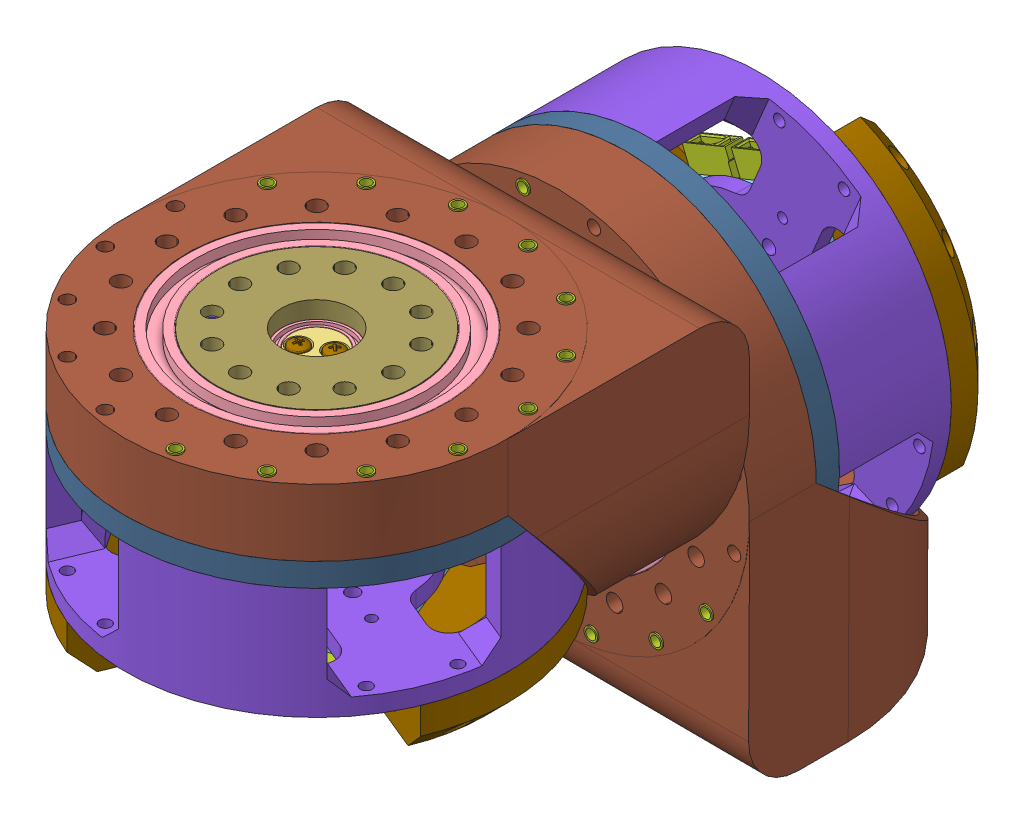
SolidWorks assembly hip, configuration Default. Lengths in mm. (continued)
Components (placement in the parent): (continued)
- Cycloidal_v3-2: Cycloidal_v3 [Default] at (91.3873 -36.6902 -47.4953) x (-0.999985 0.005457 0) z (0.005457 0.999985 0) size (150.25 88 150.25) (continued)
  - foc-motor-controller.step-1: foc-motor-controller.step [Default] at (47.267 33.7573 89.1587) x (-0.382683 0 -0.92388) z (0 -1 0) size (57.23 50 8.13) (continued)
    - RTA0040B.step-1: RTA0040B.step [Default] at (12.5014 -1.6986 1.595) x (-0.707107 -0.707107 0) z (0 0 1) size (6 6 1) (continued)
      - FRAME.step-1: FRAME.step [Default] x (1 0 0) z (0 -1 0) size (6 0.2 6) (continued)
        - SOLID-1.step-1: SOLID-1.step [Default] at origin size (0.4 0.2 0.22)
        - SOLID-2.step-1: SOLID-2.step [Default] at origin size (0.4 0.2 0.22)
        - SOLID-3.step-1: SOLID-3.step [Default] at origin size (0.4 0.2 0.22)
        - SOLID-4.step-1: SOLID-4.step [Default] at origin size (0.4 0.2 0.22)
        - SOLID-5.step-1: SOLID-5.step [Default] at origin size (0.4 0.2 0.22)
        - SOLID-6.step-1: SOLID-6.step [Default] at origin size (0.4 0.2 0.22)
        - SOLID-7.step-1: SOLID-7.step [Default] at origin size (0.4 0.2 0.22)
        - SOLID-8.step-1: SOLID-8.step [Default] at origin size (0.4 0.2 0.22)
        - SOLID-9.step-1: SOLID-9.step [Default] at origin size (0.22 0.2 0.4)
        - SOLID-10.step-1: SOLID-10.step [Default] at origin size (0.22 0.2 0.4)
        - SOLID-11.step-1: SOLID-11.step [Default] at origin size (0.22 0.2 0.4)
        - SOLID-12.step-1: SOLID-12.step [Default] at origin size (0.22 0.2 0.4)
        - SOLID-13.step-1: SOLID-13.step [Default] at origin size (0.22 0.2 0.4)
        - SOLID-14.step-1: SOLID-14.step [Default] at origin size (0.22 0.2 0.4)
        - SOLID-15.step-1: SOLID-15.step [Default] at origin size (0.22 0.2 0.4)
        - SOLID-16.step-1: SOLID-16.step [Default] at origin size (0.22 0.2 0.4)
        - SOLID-17.step-1: SOLID-17.step [Default] at origin size (4.15 0.2 4.15)
        - SOLID-18.step-1: SOLID-18.step [Default] at origin size (0.28 0.1 0.28)
        - SOLID-19.step-1: SOLID-19.step [Default] at origin size (0.28 0.1 0.28)
        - SOLID-20.step-1: SOLID-20.step [Default] at origin size (0.28 0.1 0.28)
        - SOLID-21.step-1: SOLID-21.step [Default] at origin size (0.28 0.1 0.28)
        - SOLID-22.step-1: SOLID-22.step [Default] at origin size (0.4 0.2 0.22)
        - SOLID-23.step-1: SOLID-23.step [Default] at origin size (0.4 0.2 0.22)
        - SOLID-24.step-1: SOLID-24.step [Default] at origin size (0.4 0.2 0.22)
        - SOLID-25.step-1: SOLID-25.step [Default] at origin size (0.4 0.2 0.22)
        - SOLID-26.step-1: SOLID-26.step [Default] at origin size (0.4 0.2 0.22)
        - SOLID-27.step-1: SOLID-27.step [Default] at origin size (0.4 0.2 0.22)
        - SOLID-28.step-1: SOLID-28.step [Default] at origin size (0.4 0.2 0.22)
        - SOLID-29.step-1: SOLID-29.step [Default] at origin size (0.4 0.2 0.22)
        - SOLID-30.step-1: SOLID-30.step [Default] at origin size (0.4 0.2 0.22)
        - SOLID-31.step-1: SOLID-31.step [Default] at origin size (0.4 0.2 0.22)
        - SOLID-32.step-1: SOLID-32.step [Default] at origin size (0.22 0.2 0.4)
        - SOLID-33.step-1: SOLID-33.step [Default] at origin size (0.22 0.2 0.4)
        - SOLID-34.step-1: SOLID-34.step [Default] at origin size (0.22 0.2 0.4)
        - SOLID-35.step-1: SOLID-35.step [Default] at origin size (0.22 0.2 0.4)
        - SOLID-36.step-1: SOLID-36.step [Default] at origin size (0.22 0.2 0.4)
        - SOLID-37.step-1: SOLID-37.step [Default] at origin size (0.22 0.2 0.4)
        - SOLID-38.step-1: SOLID-38.step [Default] at origin size (0.22 0.2 0.4)
        - SOLID-39.step-1: SOLID-39.step [Default] at origin size (0.22 0.2 0.4)
        - SOLID-40.step-1: SOLID-40.step [Default] at origin size (0.22 0.2 0.4)
        - SOLID-41.step-1: SOLID-41.step [Default] at origin size (0.22 0.2 0.4)
        - SOLID-42.step-1: SOLID-42.step [Default] at origin size (0.22 0.2 0.4)
        - SOLID-43.step-1: SOLID-43.step [Default] at origin size (0.22 0.2 0.4)
      - BODY.step-1: BODY.step [Default] at (0 0 0.025) x (1 0 0) z (0 -1 0) size (6 0.97 6)
    - Resonator_SMD_Murata_CSTxExxV-3Pin_3.0x1.1mm.step-1: Resonator_SMD_Murata_CSTxExxV-3Pin_3.0x1.1mm.step [Default] at (1.8 -7 1.595) x (0 1 0) z (0 0 1) size (3.2 1.35 0.9)
    - C_0603_1608Metric.step-1: C_0603_1608Metric.step [Default] at (6.2 -16.8 1.595) x (0 -1 0) z (0 0 1) size (1.6 0.8 0.8)
    - R_0603_1608Metric.step-1: R_0603_1608Metric.step [Default] at (11.8 -7.375 1.595) x (0 1 0) z (0 0 1) size (1.6 0.8 0.45)
    - R_0603_1608Metric.step-2: R_0603_1608Metric.step [Default] at (13.8 -16.8 1.595) x (0 1 0) z (0 0 1) size (1.6 0.8 0.45)
    - R_0603_1608Metric.step-3: R_0603_1608Metric.step [Default] at (18.1 -5.36 1.595) size (1.6 0.8 0.45)
    - C_0603_1608Metric.step-2: C_0603_1608Metric.step [Default] at (2.6 -0.5 1.595) x (0 -1 0) z (0 0 1) size (1.6 0.8 0.8)
    - R_0603_1608Metric.step-4: R_0603_1608Metric.step [Default] at (14.6 -11.3 1.595) x (0 1 0) z (0 0 1) size (1.6 0.8 0.45)
    - L_APV_ANR4020.step-1: L_APV_ANR4020.step [Default] at (22.3 -13.7 1.595) x (0 -1 0) z (0 0 1) size (4.02 4 2)
    - C_0603_1608Metric.step-3: C_0603_1608Metric.step [Default] at (0.3 -12.6 1.595) x (-1 0 0) z (0 0 1) size (1.6 0.8 0.8)
    - C_1206_3216Metric.step-1: C_1206_3216Metric.step [Default] at (15.7 11 1.595) x (0 1 0) z (0 0 1) size (3.2 1.6 1.6)
    - C_0603_1608Metric.step-4: C_0603_1608Metric.step [Default] at (0.3 -9.6 1.595) size (1.6 0.8 0.8)
    - R_0603_1608Metric.step-5: R_0603_1608Metric.step [Default] at (12.3 -16.8 1.595) x (0 1 0) z (0 0 1) size (1.6 0.8 0.45)
    - C_0603_1608Metric.step-5: C_0603_1608Metric.step [Default] at (-0.3 -16.6 1.595) x (0 1 0) z (0 0 1) size (1.6 0.8 0.8)
    - R_0603_1608Metric.step-6: R_0603_1608Metric.step [Default] at (10.9 4.1 1.595) size (1.6 0.8 0.45)
    - C_1206_3216Metric.step-2: C_1206_3216Metric.step [Default] at (6.3 11 1.595) x (0 1 0) z (0 0 1) size (3.2 1.6 1.6)
    - XT30PW_2_2_-M.G.B.step-1: XT30PW_2_2_-M.G.B.step [Default] at (-20.5 9.5 1.595) x (0 -1 0) z (-1 0 0) size (15.5 7.1 12.53)
    - R_0603_1608Metric.step-7: R_0603_1608Metric.step [Default] at (0.3 -11.1 1.595) size (1.6 0.8 0.45)
    - C_0603_1608Metric.step-6: C_0603_1608Metric.step [Default] at (19 -0.4 1.595) x (-0.707107 -0.707107 0) z (0 0 1) size (1.6 0.8 0.8)
    - C_1206_3216Metric.step-3: C_1206_3216Metric.step [Default] at (13.3 11 1.595) x (0 1 0) z (0 0 1) size (3.2 1.6 1.6)
    - R_0603_1608Metric.step-8: R_0603_1608Metric.step [Default] at (10.2 -7.375 1.595) x (0 -1 0) z (0 0 1) size (1.6 0.8 0.45)
    - JST_GH_SM08B-GHS-TB_1x08-1MP_P1.25mm_Horizontal.step-1: JST_GH_SM08B-GHS-TB_1x08-1MP_P1.25mm_Horizontal.step [Default] at (10 -22 1.595) size (13.25 4.95 4.25)
    - C_1206_3216Metric.step-4: C_1206_3216Metric.step [Default] at (-12.3 11 1.595) x (0 1 0) z (0 0 1) size (3.2 1.6 1.6)
    - JST_GH_SM06B-GHS-TB_1x06-1MP_P1.25mm_Horizontal.step-1: JST_GH_SM06B-GHS-TB_1x06-1MP_P1.25mm_Horizontal.step [Default] at (-4.3 -22 1.595) size (10.75 4.95 4.25)
    - C_0603_1608Metric.step-7: C_0603_1608Metric.step [Default] at (7.3 -4.5 1.595) x (-1 0 0) z (0 0 1) size (1.6 0.8 0.8)
    - R_0603_1608Metric.step-9: R_0603_1608Metric.step [Default] at (18.1 -3.86 1.595) x (-1 0 0) z (0 0 1) size (1.6 0.8 0.45)
    - C_1206_3216Metric.step-5: C_1206_3216Metric.step [Default] at (22.6794 -1.2206 1.595) x (0.707107 -0.707107 0) z (0 0 1) size (3.2 1.6 1.6)
    - R_Array_Convex_4x0402.step-1: R_Array_Convex_4x0402.step [Default] at (6.8 -2.5 1.595) size (1 2 0.35)
    - R_0603_1608Metric.step-10: R_0603_1608Metric.step [Default] at (7.7 -16.8 1.595) x (0 -1 0) z (0 0 1) size (1.6 0.8 0.45)
    - C_1206_3216Metric.step-6: C_1206_3216Metric.step [Default] at (8.7 11 1.595) x (0 1 0) z (0 0 1) size (3.2 1.6 1.6)
    - C_0603_1608Metric.step-8: C_0603_1608Metric.step [Default] at (16.1 -11.3 1.595) x (0 1 0) z (0 0 1) size (1.6 0.8 0.8)
    - SOT-23-5.step-1: SOT-23-5.step [Default] at (-3.1 -16.6 1.595) x (-1 0 0) z (0 0 1) size (2.8 2.9 1.55)
    - C_0603_1608Metric.step-9: C_0603_1608Metric.step [Default] at (17.8 -13.6 1.595) size (1.6 0.8 0.8)
    - R_0603_1608Metric.step-11: R_0603_1608Metric.step [Default] at (-11.5 -20.3875 1.595) x (0 -1 0) z (0 0 1) size (1.6 0.8 0.45)
    - C_0603_1608Metric.step-10: C_0603_1608Metric.step [Default] at (-12.4 2.3 1.595) x (0 1 0) z (0 0 1) size (1.6 0.8 0.8)
    - C_1206_3216Metric.step-7: C_1206_3216Metric.step [Default] at (18 11 1.595) x (0 1 0) z (0 0 1) size (3.2 1.6 1.6)
    - R_0603_1608Metric.step-12: R_0603_1608Metric.step [Default] at (-10.8105 -14.9971 1.595) x (-1 0 0) z (0 0 1) size (1.6 0.8 0.45)
    - C_0603_1608Metric.step-11: C_0603_1608Metric.step [Default] at (-13.8 -9.4 1.595) x (-1 0 0) z (0 0 1) size (1.6 0.8 0.8)
    - R_0603_1608Metric.step-13: R_0603_1608Metric.step [Default] at (-23.15 -14.5 1.595) x (-1 0 0) z (0 0 1) size (1.6 0.8 0.45)
    - C_0603_1608Metric.step-12: C_0603_1608Metric.step [Default] at (1.1 -0.2 1.595) x (0 1 0) z (0 0 1) size (1.6 0.8 0.8)
    - D_0805_2012Metric.step-1: D_0805_2012Metric.step [Default] at (22.9 -9.6 1.595) x (0 1 0) z (0 0 1) size (2 1.27 0.8)
    - C_0603_1608Metric.step-13: C_0603_1608Metric.step [Default] at (-7.8 3.775 1.595) x (0 -1 0) z (0 0 1) size (1.6 0.8 0.8)
    - R_0603_1608Metric.step-14: R_0603_1608Metric.step [Default] at (-6.4 -12.825 1.595) x (0 1 0) z (0 0 1) size (1.6 0.8 0.45)
    - L_0603_1608Metric.step-1: L_0603_1608Metric.step [Default] at (-10.1 3 1.595) size (1.6 0.8 0.8)
    - C_0603_1608Metric.step-14: C_0603_1608Metric.step [Default] at (17.9 0.7 1.595) x (-0.707107 -0.707107 0) z (0 0 1) size (1.6 0.8 0.8)
    - HVSSOP-10.step-1: HVSSOP-10.step [Default] at (18.6 -9.6 1.595) x (0 -1 0) z (-1 0 0) size (4.9 1.1 3)
    - C_0603_1608Metric.step-15: C_0603_1608Metric.step [Default] at (7.9 4.1 1.595) x (-1 0 0) z (0 0 1) size (1.6 0.8 0.8)
    - C_0603_1608Metric.step-16: C_0603_1608Metric.step [Default] at (21.1 -9.6 1.595) x (0 -1 0) z (0 0 1) size (1.6 0.8 0.8)
    - R_0603_1608Metric.step-15: R_0603_1608Metric.step [Default] at (-10.8105 -11.9971 1.595) x (-1 0 0) z (0 0 1) size (1.6 0.8 0.45)
    - R_0603_1608Metric.step-16: R_0603_1608Metric.step [Default] at (-18.2 -17.4 1.595) size (1.6 0.8 0.45)
    - C_1206_3216Metric.step-8: C_1206_3216Metric.step [Default] at (-3 11 1.595) x (0 1 0) z (0 0 1) size (3.2 1.6 1.6)
    - R_0603_1608Metric.step-17: R_0603_1608Metric.step [Default] at (-16.9 -20.4 1.595) x (0 -1 0) z (0 0 1) size (1.6 0.8 0.45)
    - R_0603_1608Metric.step-18: R_0603_1608Metric.step [Default] at (-13.3 -20.3875 1.595) x (0 -1 0) z (0 0 1) size (1.6 0.8 0.45)
    - R_0603_1608Metric.step-19: R_0603_1608Metric.step [Default] at (-15.1 -20.3875 1.595) x (0 -1 0) z (0 0 1) size (1.6 0.8 0.45)
    - C_0603_1608Metric.step-17: C_0603_1608Metric.step [Default] at (15.5 -14.4 1.595) x (0 -1 0) z (0 0 1) size (1.6 0.8 0.8)
    - LED_0603_1608Metric.step-1: LED_0603_1608Metric.step [Default] at (-11.5 -23.3875 1.595) x (0 1 0) z (0 0 1) size (1.6 0.8 1.1)
    - C_0805_2012Metric.step-1: C_0805_2012Metric.step [Default] at (19.95 -17 1.595) size (2 1.25 1.25)
    - D_SMB.step-1: D_SMB.step [Default] at (-16.5 11.208 1.595) x (0 -1 0) z (0 0 1) size (5.3 3.55 2.15)
    - C_1206_3216Metric.step-9: C_1206_3216Metric.step [Default] at (-5.3 11 1.595) x (0 1 0) z (0 0 1) size (3.2 1.6 1.6)
    - XT30PW_2_2_-M.G.B.step-2: XT30PW_2_2_-M.G.B.step [Default] at (-20.5 -6.5 1.595) x (0 -1 0) z (-1 0 0) size (15.5 7.1 12.53)
    - C_1206_3216Metric.step-10: C_1206_3216Metric.step [Default] at (1.7 11 1.595) x (0 1 0) z (0 0 1) size (3.2 1.6 1.6)
    - C_1206_3216Metric.step-11: C_1206_3216Metric.step [Default] at (11 11 1.595) x (0 1 0) z (0 0 1) size (3.2 1.6 1.6)
    - C_0603_1608Metric.step-18: C_0603_1608Metric.step [Default] at (-6.3 3.775 1.595) x (0 -1 0) z (0 0 1) size (1.6 0.8 0.8)
    - C_0603_1608Metric.step-19: C_0603_1608Metric.step [Default] at (16.8686 1.7314 1.595) x (0.707107 0.707107 0) z (0 0 1) size (1.6 0.8 0.8)
    - C_0603_1608Metric.step-20: C_0603_1608Metric.step [Default] at (-15.0105 -11.1 1.595) size (1.6 0.8 0.8)
    - C_1206_3216Metric.step-12: C_1206_3216Metric.step [Default] at (-7.7 11 1.595) x (0 1 0) z (0 0 1) size (3.2 1.6 1.6)
    - C_0603_1608Metric.step-21: C_0603_1608Metric.step [Default] at (-18.2 -15.8 1.595) size (1.6 0.8 0.8)
    - C_0603_1608Metric.step-22: C_0603_1608Metric.step [Default] at (-2.1 -11.3 1.595) x (0 -1 0) z (0 0 1) size (1.6 0.8 0.8)
    - C_0603_1608Metric.step-23: C_0603_1608Metric.step [Default] at (-10.8105 -13.4971 1.595) size (1.6 0.8 0.8)
    - C_1206_3216Metric.step-13: C_1206_3216Metric.step [Default] at (4 11 1.595) x (0 1 0) z (0 0 1) size (3.2 1.6 1.6)
    - R_0603_1608Metric.step-20: R_0603_1608Metric.step [Default] at (16 -17.8 1.595) x (0 1 0) z (0 0 1) size (1.6 0.8 0.45)
    - Texas_S-PVSON-N8.step-1: Texas_S-PVSON-N8.step [Default] at (-14.4105 -13.7 1.595) x (-1 0 0) z (0 0 1) size (3 2.98 0.92)
    - C_1206_3216Metric.step-14: C_1206_3216Metric.step [Default] at (21 -2.9 1.595) x (0.707107 -0.707107 0) z (0 0 1) size (3.2 1.6 1.6)
    - C_0603_1608Metric.step-24: C_0603_1608Metric.step [Default] at (-5.9 -16.6 1.595) x (0 1 0) z (0 0 1) size (1.6 0.8 0.8)
    - C_0603_1608Metric.step-25: C_0603_1608Metric.step [Default] at (-3.1 -14.1 1.595) size (1.6 0.8 0.8)
    - R_0603_1608Metric.step-21: R_0603_1608Metric.step [Default] at (7.2 -7.375 1.595) x (0 -1 0) z (0 0 1) size (1.6 0.8 0.45)
    - C_1206_3216Metric.step-15: C_1206_3216Metric.step [Default] at (-0.7 11 1.595) x (0 1 0) z (0 0 1) size (3.2 1.6 1.6)
    - LQFP-64_10x10mm_P0.5mm.step-1: LQFP-64_10x10mm_P0.5mm.step [Default] at (-7 -4.5 1.595) x (-1 0 0) z (0 0 1) size (12 12 1.5)
    - C_0805_2012Metric.step-2: C_0805_2012Metric.step [Default] at (23.35 -17 1.595) x (-1 0 0) z (0 0 1) size (2 1.25 1.25)
    - C_0603_1608Metric.step-26: C_0603_1608Metric.step [Default] at (10.8 -16.8 1.595) x (0 -1 0) z (0 0 1) size (1.6 0.8 0.8)
    - R_0603_1608Metric.step-22: R_0603_1608Metric.step [Default] at (17.5 -17.8 1.595) x (0 -1 0) z (0 0 1) size (1.6 0.8 0.45)
    - C_1206_3216Metric.step-16: C_1206_3216Metric.step [Default] at (20.3 11 1.595) x (0 1 0) z (0 0 1) size (3.2 1.6 1.6)
    - R_0603_1608Metric.step-23: R_0603_1608Metric.step [Default] at (9.2 -16.8 1.595) x (0 -1 0) z (0 0 1) size (1.6 0.8 0.45)
    - C_1206_3216Metric.step-17: C_1206_3216Metric.step [Default] at (-10 11 1.595) x (0 1 0) z (0 0 1) size (3.2 1.6 1.6)
    - R_0603_1608Metric.step-24: R_0603_1608Metric.step [Default] at (17.8 -15.2 1.595) size (1.6 0.8 0.45)
    - C_1206_3216Metric.step-18: C_1206_3216Metric.step [Default] at (19.9 2.6 1.595) x (-0.707107 0.707107 0) z (0 0 1) size (3.2 1.6 1.6)
    - C_0603_1608Metric.step-27: C_0603_1608Metric.step [Default] at (13.4 -7.375 1.595) x (0 -1 0) z (0 0 1) size (1.6 0.8 0.8)
    - R_0603_1608Metric.step-25: R_0603_1608Metric.step [Default] at (8.7 -7.375 1.595) x (0 -1 0) z (0 0 1) size (1.6 0.8 0.45)
    - PQFN-8-EP_6x5mm_P1.27mm_Generic.step-1: PQFN-8-EP_6x5mm_P1.27mm_Generic.step [Default] at (4.9 14.4 -0.085) x (0 1 0) z (0 0 -1) size (6.15 5.15 1.09)
    - C_0805_2012Metric.step-3: C_0805_2012Metric.step [Default] at (-3 8.9 -0.085) x (0 1 0) z (0 0 -1) size (2 1.25 1.25)
    - C_0603_1608Metric.step-28: C_0603_1608Metric.step [Default] at (1.5 -4.3 -0.085) x (0 1 0) z (0 0 -1) size (1.6 0.8 0.8)
    - R_2512_6332Metric.step-1: R_2512_6332Metric.step [Default] at (2.1 8.6 -0.085) x (-1 0 0) z (0 0 -1) size (6.3 3.2 0.6)
    - C_0805_2012Metric.step-4: C_0805_2012Metric.step [Default] at (18.8 8.9 -0.085) x (0 1 0) z (0 0 -1) size (2 1.25 1.25)
    - C_0805_2012Metric.step-5: C_0805_2012Metric.step [Default] at (-5.2 8.901 -0.085) x (0 1 0) z (0 0 -1) size (2 1.25 1.25)
    - PQFN-8-EP_6x5mm_P1.27mm_Generic.step-2: PQFN-8-EP_6x5mm_P1.27mm_Generic.step [Default] at (16.9 14.6 -0.085) x (0 -1 0) z (0 0 -1) size (6.15 5.15 1.09)
    - PQFN-8-EP_6x5mm_P1.27mm_Generic.step-3: PQFN-8-EP_6x5mm_P1.27mm_Generic.step [Default] at (-1.1 14.6 -0.085) x (0 -1 0) z (0 0 -1) size (6.15 5.15 1.09)
    - R_0603_1608Metric.step-26: R_0603_1608Metric.step [Default] at (8.2 8.8 -0.085) x (0 1 0) z (0 0 -1) size (1.6 0.8 0.45)
    - R_2512_6332Metric.step-2: R_2512_6332Metric.step [Default] at (-10.3 8.601 -0.085) x (1 0 0) z (0 0 -1) size (6.3 3.2 0.6)
    - TSSOP-16_4.4x5mm_P0.65mm.step-1: TSSOP-16_4.4x5mm_P0.65mm.step [Default] at (0 0 -0.085) x (-1 0 0) z (0 0 -1) size (6.4 5 1.1)
    - C_0603_1608Metric.step-29: C_0603_1608Metric.step [Default] at (0 -4.25 -0.085) x (0 1 0) z (0 0 -1) size (1.6 0.8 0.8)
    - PQFN-8-EP_6x5mm_P1.27mm_Generic.step-4: PQFN-8-EP_6x5mm_P1.27mm_Generic.step [Default] at (10.9 14.4 -0.085) x (0 1 0) z (0 0 -1) size (6.15 5.15 1.09)
    - R_2512_6332Metric.step-3: R_2512_6332Metric.step [Default] at (13.7 8.6 -0.085) x (1 0 0) z (0 0 -1) size (6.3 3.2 0.6)
    - PQFN-8-EP_6x5mm_P1.27mm_Generic.step-5: PQFN-8-EP_6x5mm_P1.27mm_Generic.step [Default] at (-13.1 14.401 -0.085) x (0 1 0) z (0 0 -1) size (6.15 5.15 1.09)
    - C_0603_1608Metric.step-30: C_0603_1608Metric.step [Default] at (-1.5 -4.3 -0.085) x (0 -1 0) z (0 0 -1) size (1.6 0.8 0.8)
    - PQFN-8-EP_6x5mm_P1.27mm_Generic.step-6: PQFN-8-EP_6x5mm_P1.27mm_Generic.step [Default] at (-7.1 14.601 -0.085) x (0 -1 0) z (0 0 -1) size (6.15 5.15 1.09)
    - foc-motor-controller_PCB.step-1: foc-motor-controller_PCB.step [Default] at origin size (50 50 1.51)
  - hex nut style 1 gradeab_iso-1: hex nut style 1 gradeab_iso [ISO - 4032 - M3 - W - N] at (35.6313 33.7573 117.2498) x (1 0 0) z (0 -1 0) size (5.5 6.35 2.4)
  - Cycloidal_Discs_8308-1: Cycloidal_Discs_8308 [Default] at (6.9481 42.227 30.6143) x (0.999764 0 -0.021738) z (0.021738 0 0.999764) size (79.25 5 79.73)
    - Cycloidal_Discs-1: Cycloidal_Discs [Default] at (38.3081 39.5303 58.0959) size (79.25 5 79.73)
    - radial ball bearing_68_iso-1: radial ball bearing_68_iso [ISO 15 RBB - 274 - 14,SI,NC,14_68] at (18.3896 43.2803 46.5959) x (0 1 0) z (0 0 1) size (2.5 7 7)
    - radial ball bearing_68_iso-2: radial ball bearing_68_iso [ISO 15 RBB - 274 - 14,SI,NC,14_68] at (38.3081 43.2803 81.0959) x (0 1 0) z (0 0 1) size (2.5 7 7)
    - radial ball bearing_68_iso-3: radial ball bearing_68_iso [ISO 15 RBB - 274 - 14,SI,NC,14_68] at (18.3896 43.2803 69.5959) x (0 1 0) z (0 0 1) size (2.5 7 7)
    - radial ball bearing_68_iso-4: radial ball bearing_68_iso [ISO 15 RBB - 274 - 14,SI,NC,14_68] at (38.3081 43.2803 35.0959) x (0 1 0) z (0 0 1) size (2.5 7 7)
    - radial ball bearing_68_iso-5: radial ball bearing_68_iso [ISO 15 RBB - 274 - 14,SI,NC,14_68] at (58.2267 43.2803 69.5959) x (0 1 0) z (0 0 1) size (2.5 7 7)
    - radial ball bearing_68_iso-6: radial ball bearing_68_iso [ISO 15 RBB - 274 - 14,SI,NC,14_68] at (58.2267 43.2803 46.5959) x (0 1 0) z (0 0 1) size (2.5 7 7)
  - Cycloidal_Discs_8308-2: Cycloidal_Discs_8308 [Default] at (85.7348 37.227 31.9683) x (0.403317 0 0.91506) z (-0.91506 0 0.403317) size (79.25 5 79.73)
    - Cycloidal_Discs-1: Cycloidal_Discs [Default] at (38.3081 39.5303 58.0959) size (79.25 5 79.73)
    - radial ball bearing_68_iso-1: radial ball bearing_68_iso [ISO 15 RBB - 274 - 14,SI,NC,14_68] at (18.3896 43.2803 46.5959) x (0 1 0) z (0 0 1) size (2.5 7 7)
    - radial ball bearing_68_iso-2: radial ball bearing_68_iso [ISO 15 RBB - 274 - 14,SI,NC,14_68] at (38.3081 43.2803 81.0959) x (0 1 0) z (0 0 1) size (2.5 7 7)
    - radial ball bearing_68_iso-3: radial ball bearing_68_iso [ISO 15 RBB - 274 - 14,SI,NC,14_68] at (18.3896 43.2803 69.5959) x (0 1 0) z (0 0 1) size (2.5 7 7)
    - radial ball bearing_68_iso-4: radial ball bearing_68_iso [ISO 15 RBB - 274 - 14,SI,NC,14_68] at (38.3081 43.2803 35.0959) x (0 1 0) z (0 0 1) size (2.5 7 7)
    - radial ball bearing_68_iso-5: radial ball bearing_68_iso [ISO 15 RBB - 274 - 14,SI,NC,14_68] at (58.2267 43.2803 69.5959) x (0 1 0) z (0 0 1) size (2.5 7 7)
    - radial ball bearing_68_iso-6: radial ball bearing_68_iso [ISO 15 RBB - 274 - 14,SI,NC,14_68] at (58.2267 43.2803 46.5959) x (0 1 0) z (0 0 1) size (2.5 7 7)
  - m6-1: m6 [Default] at (27.3484 93.9895 100.6587) x (-0.80367 0 -0.595076) z (-0.595076 0 0.80367) size (6 16 6)
  - Motor_Cover_v2-2: Motor_Cover_v2 [Default] at (47.267 36.1573 89.1587) x (-0.92388 0 -0.382683) z (0.382683 0 -0.92388) size (115 33.6 115)
  - driver_cover-1: driver_cover [Default] at (47.267 36.1573 89.1587) x (-0.384295 0 -0.92321) z (-0.92321 0 0.384295) size (81.32 15 115)
  - Base_plate_2-1: Base_plate_2 [Default] at (47.267 69.7573 89.1587) size (115 7 115)
  - Cover_new-1: Cover_new [Default] at (47.267 86.8173 89.1587) size (115 87.56 130)
  - Output_Shaft-1: Output_Shaft [Default] at (47.267 86.8173 89.1587) size (60 10 60)
Mates (geometry in assembly coordinates):
- Coincident1: coincident anti-aligned: plane of Cycloidal_v3-1/Cover_new-1 through (102.1075 100.2851 49.3221) normal (0 0 -1); plane of Cycloidal_v3-2/Output_Shaft-1 through (44.6075 52.7251 49.3221) normal (0 0 1)
- Concentric2: concentric: cylinder of Cycloidal_v3-1/Cover_new-1 through (56.1075 72.6437 116.8221) axis (0 0 -1) radius 2; cylinder of Cycloidal_v3-2/Output_Shaft-1 through (56.1075 72.6437 49.3221) axis (0 0 -1) radius 2.5
- Concentric5: concentric: cylinder of Cycloidal_v3-1/Cover_new-1 through (56.1075 32.8065 116.8221) axis (0 0 -1) radius 2; cylinder of Cycloidal_v3-2/Output_Shaft-1 through (56.1075 32.8065 49.3221) axis (0 0 -1) radius 2.5
